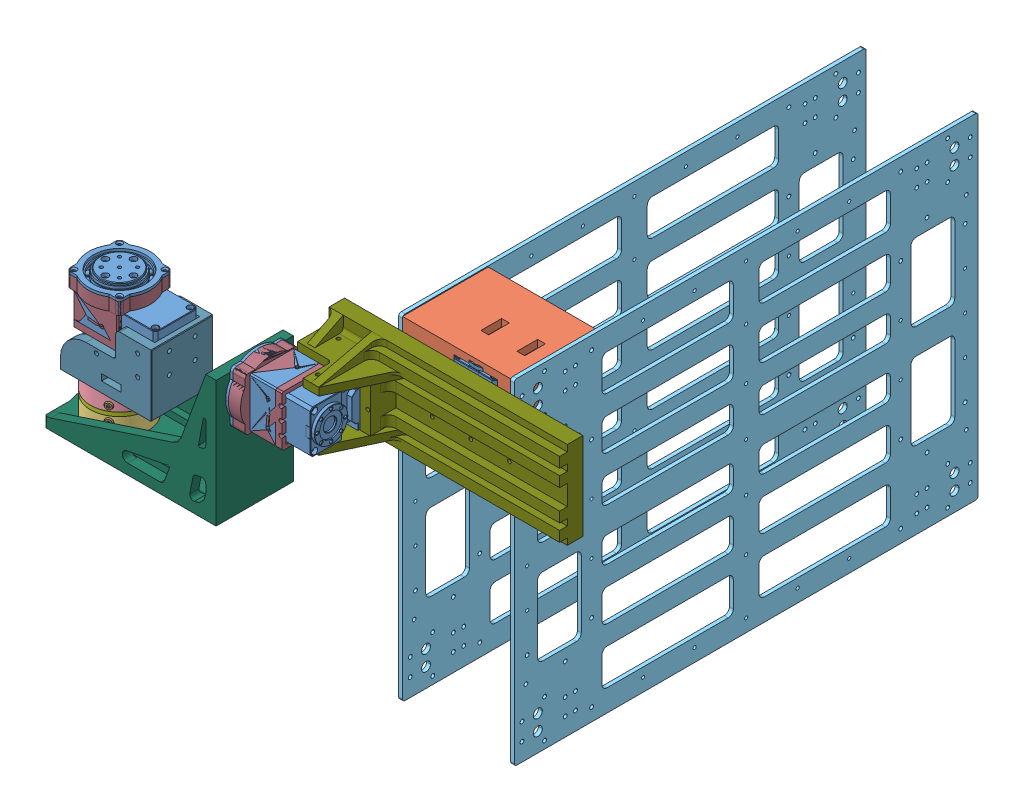
SolidWorks assembly 单轮-1, configuration Default. Lengths in mm.
Overall size (333.74 260 458.54).
45 component instances, 24 part files, 41 mates.
Components (placement in the parent):
- 540总装-1: 540总装 [默认] at (-9.2345 7.2685 42.6291) size (68.75 59.5 48)
- 透明车轮-加工版-1: 透明车轮-加工版 [默认] at (4.5155 78.2685 59.3791) x (0.291956 0 0.956432) z (0 -1 0) size (149.62 149.62 76) (hidden)
- 3813d-00_asm-2.0-1: 3813d-00_asm-2.0 [默认] at (4.5155 -18.8315 59.3791) x (0.5 0 0.866025) z (0 -1 0) size (46.1 51.16 31)
  - 3813d-00_asm.stp-1: 3813d-00_asm.stp [默认] at origin size (46.1 51.16 31)
    - 3813D-00_ASM_99_ASM.stp-1: 3813D-00_ASM_99_ASM.stp [默认] at origin size (46.1 51.16 31)
      - 3813D-10_ASM_33_ASM.stp-1: 3813D-10_ASM_33_ASM.stp [默认] at origin size (39.84 42 29.09)
        - 3813D-15_181.stp-1: 3813D-15_181.stp [Default] at origin size (39.84 42 29.01)
      - 3813D-26_48.stp-1: 3813D-26_48.stp [默认] at (0 0 1.5) size (45 45 13.8)
      - 38133-27_40.stp-1: 38133-27_40.stp [默认] at (0 0 -1.5) x (1 0 0) z (0 0 -1) size (45 45 13.8)
      - 38133-29_43.stp-1: 38133-29_43.stp [Default] at (0 0 -14.5) x (1 0 0) z (0 0 -1) size (42 42 1)
      - 38133-FILLER1_6.stp-1: 38133-FILLER1_6.stp [默认] at (0 0 -15.5) size (44 44 1)
      - 38133-FILLER2_5.stp-1: 38133-FILLER2_5.stp [默认] at (0 0 -1.5) size (45 45 3)
      - 5000595_22.stp-1: 5000595_22.stp [默认] at (-9 0 -15.5) x (0 0 1) z (0 1 0) size (4.01 4 4)
      - 5000595_22.stp-2: 5000595_22.stp [默认] at (4.5 7.7942 -15.5) x (0 0 1) z (0 1 0) size (4.01 4 4)
      - 5000595_22.stp-3: 5000595_22.stp [默认] at (4.5 -7.7942 -15.5) x (0 0 1) z (0 1 0) size (4.01 4 4)
      - 38133-29_43.stp-2: 38133-29_43.stp [Default] at (0 0 14.5) size (42 42 1)
      - 38133-FILLER1_6.stp-2: 38133-FILLER1_6.stp [默认] at (0 0 14.5) size (44 44 1)
      - 38133-31_31.stp-1: 38133-31_31.stp [默认] at (5.15 -8.9201 -11.5) x (0 0 1) z (0.5 -0.866025 0) size (6.5 15 11.5)
      - 5000456_66.stp-1: 5000456_66.stp [默认] at (4.3869 -18.5983 -11.5) x (0.866025 0.5 0) z (0.5 -0.866025 0) size (4.5 4.5 12.51)
      - 5000456_66.stp-2: 5000456_66.stp [默认] at (13.9131 -13.0983 -11.5) x (0.866025 0.5 0) z (0.5 -0.866025 0) size (4.5 4.5 12.51)
      - 38133-CABLE_4.stp-1: 38133-CABLE_4.stp [默认] at (8.4 -14.5492 -11.5) x (0.866025 0.5 0) z (0.5 -0.866025 0) size (4.5 4.5 15)
      - 5000429_2.stp-1: 5000429_2.stp [默认] at (22 0 -5.5) x (0 -1 0) z (-1 0 0) size (5.5 5.5 6.61)
      - 5000429_2.stp-2: 5000429_2.stp [默认] at (-11 -19.0526 -5.5) x (-0.866025 0.5 0) z (0.5 0.866025 0) size (5.5 5.5 6.61)
      - 5000429_2.stp-3: 5000429_2.stp [默认] at (-11 19.0526 -5.5) x (0.866025 0.5 0) z (0.5 -0.866025 0) size (5.5 5.5 6.61)
      - 5000429_2.stp-4: 5000429_2.stp [默认] at (22 0 5.5) x (0 -1 0) z (-1 0 0) size (5.5 5.5 6.61)
      - 5000429_2.stp-5: 5000429_2.stp [默认] at (-11 19.0526 5.5) x (0.866025 0.5 0) z (0.5 -0.866025 0) size (5.5 5.5 6.61)
      - 5000429_2.stp-6: 5000429_2.stp [默认] at (-11 -19.0526 5.5) x (-0.866025 0.5 0) z (0.5 0.866025 0) size (5.5 5.5 6.61)
      - 5000595_22.stp-4: 5000595_22.stp [默认] at (-9 0 15.5) x (0 0 -1) z (0 1 0) size (4.01 4 4)
      - 5000595_22.stp-5: 5000595_22.stp [默认] at (4.5 -7.7942 15.5) x (0 0 -1) z (0 1 0) size (4.01 4 4)
      - 5000595_22.stp-6: 5000595_22.stp [默认] at (4.5 7.7942 15.5) x (0 0 -1) z (0 1 0) size (4.01 4 4)
- 外壳.step-1: 外壳.step [默认] at (-9.2345 51.2685 76.1291) x (0 0 -1) z (0 -1 0) size (48 48 34.5)
- 方案2-大L-1: 方案2-大L [Default] at (39.3905 4.6685 59.3791) x (0 0 -1) z (1 0 0) size (47.8 48 70.75)
- L连接-1: L连接 [Default] at (4.5155 -42.3315 29.3791) x (0 0 1) z (0 1 0) size (60 135 98)
- 540总装-2: 540总装 [默认] at (166.5155 23.5185 73.1291) x (0 0 -1) z (0 1 0) size (68.75 59.5 48)
- 外壳.step-2: 外壳.step [默认] at (122.5155 57.0185 73.1291) x (0 -1 0) z (1 0 0) size (48 48 34.5)
- 新的升降台v4-1: 新的升降台v4 [Default] at (307.5155 6.3685 2.6291) x (0 -1 0) z (0 0 1) size (67.8 185 66)
- HIWIN Corporation-MGWR-9-R0500-1: HIWIN Corporation-MGWR-9-R0500 [Default] at (201.7296 40.2685 1.0299) x (0 -1 0) z (1 0 0) size (17 7 120)
- 齿条.step-1: 齿条.step [默认] at (205.1472 22.5685 10.7791) x (1 0 0) z (0 1 0) size (90 11 10)
- 模块化移动导轨-1: 模块化移动导轨 [Default] at (243.9058 53.6652 -27.233) x (1 0 0) z (0 -1 0) size (83.8 75.6 65)
  - 540舵机-1: 540舵机 [默认] at (-29.5731 8.012 7.2851) size (33.51 58.5 54.3)
  - 模块-方案2-1: 模块-方案2 [Default] at (48.5269 19.762 -30.5649) x (0 -1 0) z (0 0 1) size (66.5 83.8 65)
  - HIWIN Corporation-MGW-9C-1: HIWIN Corporation-MGW-9C [Default] at (-54.7465 30.8042 16.0803) x (0 0 -1) z (-1 0 0) size (30 9.1 39.26)
- 齿轮.step-1: 齿轮.step [默认] at (214.3327 13.8801 -19.2209) x (0 1 0) z (0.985048 0 0.172277) size (8 41.91 41.91)
- 上底板切割-1: 上底板切割 [默认] at (244.2327 -55.0699 -187.4709) x (0 0 1) z (-1 0 0) size (360 260 3)
- 上底板切割-2: 上底板切割 [默认] at (157.4327 -55.0699 -187.4709) x (0 0 1) z (-1 0 0) size (360 260 3)
Mates (geometry in assembly coordinates):
- 同心1: concentric anti-aligned: cylinder of 540总装-1 through (4.5155 62.7685 59.3791) axis (0 -1 0) radius 16; cylinder of 透明车轮-加工版-1 through (4.5155 2.2685 59.3791) axis (0 1 0) radius 5.05
- 重合1: coincident anti-aligned: plane of 540总装-1 through (4.5155 64.2685 59.3791) normal (0 1 0); plane of 透明车轮-加工版-1 through (4.5155 64.2685 59.3791) normal (0 -1 0)
- 同心2: concentric anti-aligned: cylinder of 540总装-1 through (4.5155 7.3935 59.3791) axis (0 -1 0) radius 5; cylinder of 3813d-00_asm-2.0-1/3813d-00_asm.stp-1/3813D-00_ASM_99_ASM.stp-1/38133-27_40.stp-1 through (4.5155 -17.3315 59.3791) axis (0 1 0) radius 22.5
- 重合5: coincident aligned: plane of 540总装-1 through (-9.2345 51.2685 76.1291) normal (0 -1 0); plane of 外壳.step-1 through (-9.2345 51.2685 76.1291) normal (0 -1 0)
- 同心7: concentric aligned: cylinder of 540总装-1 through (4.5155 7.3935 59.3791) axis (0 -1 0) radius 5; circle of 外壳.step-1
- 同心11: concentric aligned: cylinder of 3813d-00_asm-2.0-1/3813d-00_asm.stp-1/3813D-00_ASM_99_ASM.stp-1/3813D-10_ASM_33_ASM.stp-1/3813D-15_181.stp-1 through (4.5155 -33.3315 59.3791) axis (0 1 0) radius 4.01; cylinder of 方案2-大L-1 through (4.5155 -3.3315 59.3791) axis (0 1 0) radius 4.125
- 同心12: concentric anti-aligned: cylinder of 3813d-00_asm-2.0-1/3813d-00_asm.stp-1/3813D-00_ASM_99_ASM.stp-1/3813D-10_ASM_33_ASM.stp-1/3813D-15_181.stp-1 through (12.5155 -21.7905 45.5227) axis (0 -1 0) radius 1.65; cylinder of 方案2-大L-1 through (12.5155 4.6685 45.5227) axis (0 1 0) radius 2.25
- 重合11: coincident anti-aligned: plane of 3813d-00_asm-2.0-1/3813d-00_asm.stp-1/3813D-00_ASM_99_ASM.stp-1/38133-29_43.stp-1 through (4.5155 -3.3315 59.3791) normal (0 1 0); plane of 方案2-大L-1 through (39.3905 -3.3315 59.3791) normal (0 -1 0)
- 平行4: parallel aligned: plane of 540总装-1 through (49.2655 7.2685 76.1291) normal (1 0 0); plane of 方案2-大L-1 through (53.2655 44.6685 59.3791) normal (1 0 0)
- 同心13: concentric aligned: cylinder of 540总装-1 through (42.5155 37.2685 72.3324) axis (0 0 -1) radius 1.025; cylinder of 方案2-大L-1 through (42.5155 37.2685 80.2791) axis (0 0 -1) radius 1.6
- 同心14: concentric aligned: cylinder of 540总装-1 through (10.5155 37.2685 79.1291) axis (0 0 -1) radius 1.5; cylinder of 外壳.step-1 through (10.5155 37.2685 79.1291) axis (0 0 -1) radius 1.5
- 同心15: concentric aligned: cylinder of 3813d-00_asm-2.0-1/3813d-00_asm.stp-1/3813D-00_ASM_99_ASM.stp-1/3813D-10_ASM_33_ASM.stp-1/3813D-15_181.stp-1 through (9.0155 -33.3315 67.1733) axis (0 1 0) radius 1.51; cylinder of 方案2-大L-1 through (9.0155 -3.3315 67.1733) axis (0 1 0) radius 1.625
- 同心16: concentric aligned: cylinder of 3813d-00_asm-2.0-1/3813d-00_asm.stp-1/3813D-00_ASM_99_ASM.stp-1/3813D-26_48.stp-1 through (4.5155 -20.3315 59.3791) axis (0 -1 0) radius 22.5; cylinder of L连接-1 through (4.5155 -34.3315 59.3791) axis (0 -1 0) radius 30
- 重合12: coincident anti-aligned: plane of 3813d-00_asm-2.0-1/3813d-00_asm.stp-1/3813D-00_ASM_99_ASM.stp-1/38133-29_43.stp-2 through (4.5155 -34.3315 59.3791) normal (0 -1 0); plane of L连接-1 through (4.5155 -34.3315 29.3791) normal (0 1 0)
- 同心17: concentric anti-aligned: cylinder of 3813d-00_asm-2.0-1/3813d-00_asm.stp-1/3813D-00_ASM_99_ASM.stp-1/3813D-10_ASM_33_ASM.stp-1/3813D-15_181.stp-1 through (9.0155 -33.3315 67.1733) axis (0 1 0) radius 1.51; cylinder of L连接-1 through (9.0155 -34.3315 67.1733) axis (0 -1 0) radius 1.625
- 同心18: concentric aligned: cylinder of 540总装-2 through (109.5155 40.2685 59.3791) axis (1 0 0) radius 15; cylinder of 外壳.step-2 through (112.5155 40.2685 59.3791) axis (1 0 0) radius 14
- 重合13: coincident anti-aligned: plane of 540总装-2 through (122.5155 40.2685 59.3791) normal (-1 0 0); plane of 外壳.step-2 through (122.5155 57.0185 73.1291) normal (1 0 0)
- 同心19: concentric aligned: cylinder of 540总装-2 through (136.5155 30.2685 73.1291) axis (0 0 1) radius 1.5; cylinder of 外壳.step-2 through (136.5155 30.2685 73.1291) axis (0 0 1) radius 1.5
- 重合14: coincident anti-aligned: plane of L连接-1 through (109.5155 -34.3315 29.3791) normal (1 0 0); plane of 540总装-2 through (109.5155 40.2685 59.3791) normal (-1 0 0)
- 同心22: concentric anti-aligned: cylinder of L连接-1 through (39.5155 40.2685 59.3791) axis (1 0 0) radius 1.6; cylinder of 540总装-2 through (109.5155 40.2685 59.3791) axis (-1 0 0) radius 1.25
- 重合16: coincident anti-aligned: plane of 540总装-2 through (166.5155 57.0185 14.6291) normal (0 0 -1); plane of 新的升降台v4-1 through (307.5155 6.3685 14.6291) normal (0 0 1)
- 同心23: concentric anti-aligned: cylinder of 540总装-2 through (136.5155 50.2685 18.4258) axis (0 0 -1) radius 1.025; cylinder of 新的升降台v4-1 through (136.5155 50.2685 -1.4721) axis (0 0 1) radius 1.45
- 同心24: concentric anti-aligned: cylinder of 540总装-2 through (136.5155 30.2685 18.4258) axis (0 0 -1) radius 1.025; cylinder of 新的升降台v4-1 through (136.5155 30.2685 -1.4721) axis (0 0 1) radius 1.45
- 平行6: parallel aligned: plane of 新的升降台v4-1 through (307.5155 6.3685 2.6291) normal (0 0 -1); plane of L连接-1 through (4.5155 -34.3315 29.3791) normal (0 0 -1)
- 重合20: coincident anti-aligned: plane of 新的升降台v4-1 through (307.5155 6.3685 10.7791) normal (0 0 -1); plane of 齿条.step-1 through (205.1472 12.5685 10.7791) normal (0 0 1)
- 重合22: coincident anti-aligned: plane of 新的升降台v4-1 through (307.5155 12.5685 10.7791) normal (0 1 0); plane of 齿条.step-1 through (205.1472 12.5685 -0.2209) normal (0 -1 0)
- 平行7: parallel anti-aligned: plane of 新的升降台v4-1 through (307.5155 6.3685 2.6291) normal (0 0 -1); plane of 模块化移动导轨-1/模块-方案2-1 through (187.4327 24.2301 -7.4709) normal (0 0 1)
- 同心25: concentric anti-aligned: cylinder of 模块化移动导轨-1/540舵机-1 through (214.3327 19.1301 -19.2209) axis (0 1 0) radius 5; cylinder of 齿轮.step-1 through (214.3327 33.8801 -19.2209) axis (0 -1 0) radius 5.2
- 重合25: coincident anti-aligned: plane of 模块化移动导轨-1/540舵机-1 through (214.3327 21.8801 -19.2209) normal (0 -1 0); plane of 齿轮.step-1 through (214.3327 21.8801 -19.2209) normal (0 1 0)
- 同心26: concentric aligned: cylinder of HIWIN Corporation-MGWR-9-R0500-1 through (451.7296 31.9685 -0.2709) axis (-1 0 0) radius 0.35; cylinder of 模块化移动导轨-1/HIWIN Corporation-MGW-9C-1 through (197.1964 31.9685 -0.2709) axis (-1 0 0) radius 0.35
- 距离2: distance = 30 mm: plane of 新的升降台v4-1 through (307.5155 6.3685 10.7791) normal (0 0 -1); cylinder of 齿轮.step-1 through (214.3327 33.8801 -19.2209) axis (0 -1 0) radius 5.2
- 平行8: parallel aligned: plane of 新的升降台v4-1 through (307.5155 6.3685 14.6291) normal (1 0 0); plane of HIWIN Corporation-MGWR-9-R0500-1 through (277.5155 40.2685 7.5299) normal (1 0 0)
- 平行9: parallel aligned: plane of 新的升降台v4-1 through (307.5155 6.3685 2.6291) normal (0 0 -1); plane of HIWIN Corporation-MGWR-9-R0500-1 through (451.7296 31.7677 -2.4701) normal (0 0 -1)
- 同心27: concentric aligned: cylinder of 新的升降台v4-1 through (172.5155 40.2685 2.6291) axis (0 0 -1) radius 1.45; cylinder of HIWIN Corporation-MGWR-9-R0500-1 through (172.5155 40.2685 -2.4701) axis (0 0 -1) radius 3
- 重合26: coincident anti-aligned: plane of 模块化移动导轨-1/模块-方案2-1 through (241.2327 84.2301 -7.4709) normal (1 0 0); plane of 上底板切割-1 through (241.2327 -55.0699 -187.4709) normal (-1 0 0)
- 重合27: coincident anti-aligned: plane of 模块化移动导轨-1/模块-方案2-1 through (157.4327 84.2301 -73.4709) normal (-1 0 0); plane of 上底板切割-2 through (157.4327 -55.0699 -187.4709) normal (1 0 0)
- 重合28: coincident aligned: plane of 上底板切割-1 through (241.2327 -185.0699 -7.4709) normal (0 0 1); plane of 上底板切割-2 through (154.4327 -185.0699 -7.4709) normal (0 0 1)
- 重合29: coincident aligned: plane of 上底板切割-1 through (241.2327 -185.0699 -367.4709) normal (0 -1 0); plane of 上底板切割-2 through (154.4327 -185.0699 -367.4709) normal (0 -1 0)
- 同心28: concentric anti-aligned: cylinder of 模块化移动导轨-1/模块-方案2-1 through (241.2327 47.6301 -13.4709) axis (1 0 0) radius 1.45; cylinder of 上底板切割-1 through (251.2327 47.6301 -13.4709) axis (-1 0 0) radius 1.5
- 平行11: parallel anti-aligned: cylinder of 模块化移动导轨-1/模块-方案2-1 through (241.2327 60.8801 -54.9702) axis (1 0 0) radius 1.45; cylinder of 上底板切割-1 through (251.2327 60.9301 -54.9709) axis (-1 0 0) radius 1.5
- 同心33: concentric anti-aligned: cylinder of 模块化移动导轨-1/模块-方案2-1 through (241.2327 69.1301 -30.9709) axis (1 0 0) radius 1.45; cylinder of 上底板切割-1 through (251.2327 69.1301 -30.9709) axis (-1 0 0) radius 1.5
